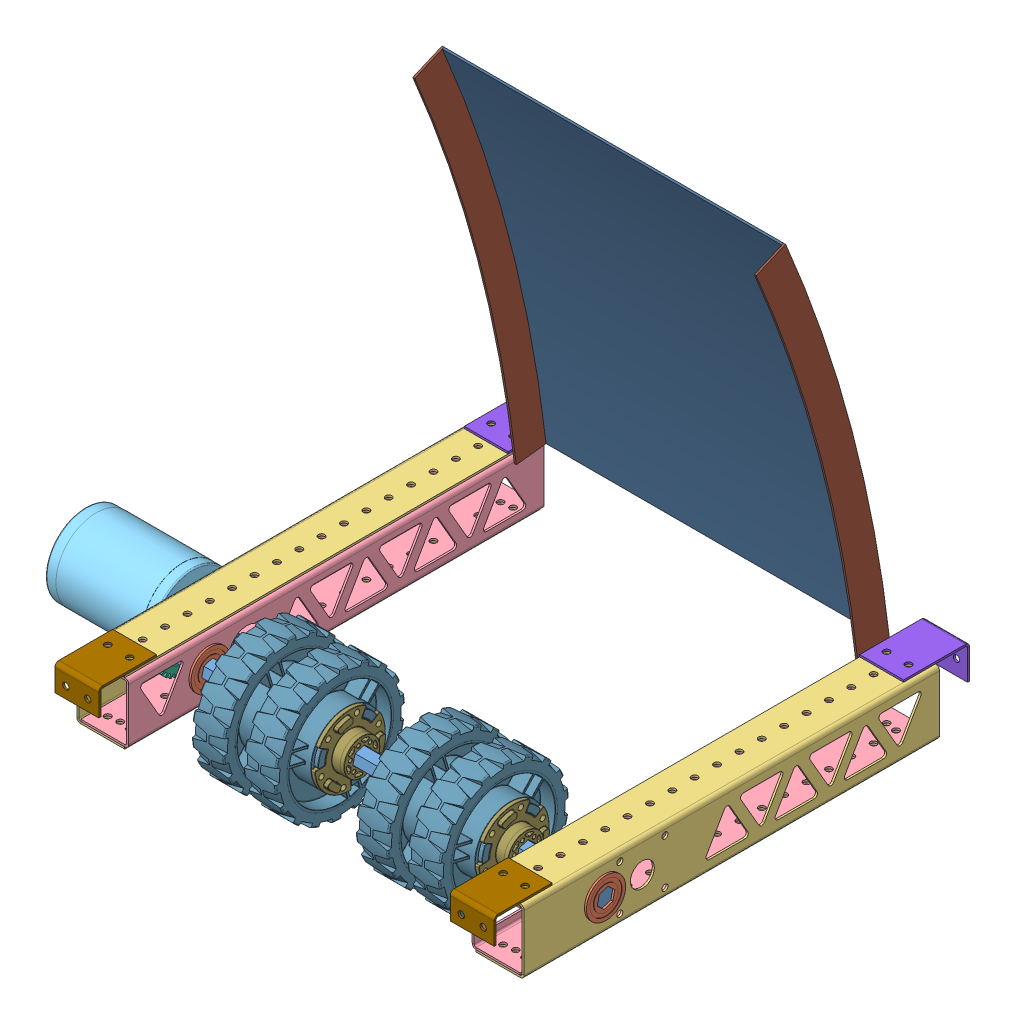
SolidWorks assembly 0001 - 03 - 1001 REVISED SHOOTER, configuration Default. Lengths in mm.
34 component instances, 15 part files, 27 mates.
Components (placement in the parent):
- 0001 - 03 - 1000 SHOOTER-1: 0001 - 03 - 1000 SHOOTER [Default] at (243.3681 260.9719 308.2005) size (448.99 90.52 330.2)
  - 0001 - 03 - 0001 Reference Geometry-1: 0001 - 03 - 0001 Reference Geometry [Default] at origin
  - 0001 - 03 - 1011 Hex Shaft-1: 0001 - 03 - 1011 Hex Shaft [Default] at (158.75 29.2246 103.7425) x (1 0 0) z (0 -0.904809 0.425818) size (355.6 13.95 14.34)
  - Hex Bearing-4: Hex Bearing [Default] at (330.2 0 101.6) x (0 -0.973926 0.226866) z (0 0.226866 0.973926) size (31.12 7.94 31.12)
  - Hex Bearing-5: Hex Bearing [Default] at (301.625 0 101.6) x (0 0.290491 -0.956878) z (0 0.956878 0.290491) size (31.12 7.94 31.12)
  - 0001 - 03 - 1023 Left Side-1: 0001 - 03 - 1023 Left Side [Default] x (0 0 1) z (-1 0 0) size (330.2 50.8 38.1)
  - 0001 - 03 - 1022 Right Side-1: 0001 - 03 - 1022 Right Side [Default] at (2.3813 0 0) x (0 0 -1) z (1 0 0) size (330.2 47.62 38.1)
  - 0001 - 03 - 1022 Right Side-2: 0001 - 03 - 1022 Right Side [Default] at (315.1187 0 0) x (0 0 -1) z (-1 0 0) size (330.2 47.62 38.1)
  - 0001 - 03 - 1023 Left Side-2: 0001 - 03 - 1023 Left Side [Default] at (317.5 0 0) x (0 0 1) z (1 0 0) size (330.2 50.8 38.1)
  - Mini-CIM-2: Mini-CIM [Default] at (-20.6375 0 71.12) x (-1 0 0) z (0 -0.707107 0.707107) size (125.82 64.01 64.01)
  - Hex Bearing-6: Hex Bearing [Default] at (-12.7 0 101.6) x (0 -0.973926 0.226866) z (0 -0.226866 -0.973926) size (31.12 7.94 31.12)
  - Hex Bearing-7: Hex Bearing [Default] at (15.875 0 101.6) x (0 0.973926 -0.226866) z (0 -0.226866 -0.973926) size (31.12 7.94 31.12)
  - 24t Vex Gear-1: 24t Vex Gear [Default] at (-6.3754 0 71.12) x (0 -0.442832 0.896605) z (-1 0 0) size (32.86 32.86 12.65)
  - 24t Vex Gear-2: 24t Vex Gear [Default] at (-6.3754 0 101.6) x (0 -0.944341 0.328968) z (-1 0 0) size (32.86 32.86 12.65)
  - CIM Shaft Adapter-1: CIM Shaft Adapter [Default] at (-16.6375 0 71.12) x (1 0 0) z (0 0.064799 0.997898) size (19.05 12.7 14.66)
- 0001 - 03 - 1024 Bracket-1: 0001 - 03 - 1024 Bracket [Default] at (244.9556 260.9719 117.7005) x (-1 0 0) z (0 0 -1) size (34.92 26.99 52.39)
- 0001 - 03 - 1024 Bracket-2: 0001 - 03 - 1024 Bracket [Default] at (559.2806 260.9719 117.7005) x (-1 0 0) z (0 0 -1) size (34.92 26.99 52.39)
- 0001 - 03 - 1025 Small Bracket-1: 0001 - 03 - 1025 Small Bracket [Default] at (244.9556 267.3219 492.3505) size (34.92 20.64 46.04)
- 0001 - 03 - 1025 Small Bracket-2: 0001 - 03 - 1025 Small Bracket [Default] at (559.2806 267.3219 492.3505) size (34.92 20.64 46.04)
- 0001 - 03 - 1026 Hood-1: 0001 - 03 - 1026 Hood [Default] at (537.0556 283.3795 141.5236) x (-1 0 0) z (0 0.115024 -0.993363) size (269.88 320.68 47.56)
- 0001 - 03 - 1027 Hood Support-1: 0001 - 03 - 1027 Hood Support [Default] at (267.1806 596.6307 224.1409) x (1 0 0) z (0 0.389841 -0.920882) size (1.59 320.68 70.41)
- 0001 - 03 - 1027 Hood Support-2: 0001 - 03 - 1027 Hood Support [Default] at (538.6431 596.6307 224.1409) x (1 0 0) z (0 0.389841 -0.920882) size (1.59 320.68 70.41)
- 0001 - 03 - 1030 WHEEL ASSEMBLY-1: 0001 - 03 - 1030 WHEEL ASSEMBLY [Default] at (328.3429 264.0107 383.1758) x (0 0.956878 0.290491) z (1 0 0) size (140.96 140.96 101.35)
  - VersaHub-1: VersaHub [Default] at (4.8265 26.3593 48.1847) size (54.75 55.87 12.7)
  - VersaThing-1: VersaThing [Default] at (4.8265 26.3593 8.6242) x (-0.5 0.866025 0) z (0.866025 0.5 0) size (55.88 12.7 55.88)
  - VEX Wheel 4in DT-1: VEX Wheel 4in DT [Default] at (4.8265 26.3593 29.1982) x (0.5 -0.866025 0) z (0 0 1) size (103.19 103.19 41.15)
  - VersaHub-2: VersaHub [Default] at (4.8265 26.3593 -30.9363) x (-0.5 -0.866025 0) z (0 0 -1) size (54.75 55.87 12.7)
  - VEX Wheel 4in DT-2: VEX Wheel 4in DT [Default] at (4.8265 26.3593 -11.9498) size (103.19 103.19 41.15)
- 0001 - 03 - 1030 WHEEL ASSEMBLY-2: 0001 - 03 - 1030 WHEEL ASSEMBLY [Default] at (475.8933 246.4805 387.2593) x (0 -0.730012 0.683435) z (-1 0 0) size (140.96 140.96 101.35)
  - VersaHub-1: VersaHub [Default] at (4.8265 26.3593 48.1847) size (54.75 55.87 12.7)
  - VersaThing-1: VersaThing [Default] at (4.8265 26.3593 8.6242) x (-0.5 0.866025 0) z (0.866025 0.5 0) size (55.88 12.7 55.88)
  - VEX Wheel 4in DT-1: VEX Wheel 4in DT [Default] at (4.8265 26.3593 29.1982) x (0.5 -0.866025 0) z (0 0 1) size (103.19 103.19 41.15)
  - VersaHub-2: VersaHub [Default] at (4.8265 26.3593 -30.9363) x (-0.5 -0.866025 0) z (0 0 -1) size (54.75 55.87 12.7)
  - VEX Wheel 4in DT-2: VEX Wheel 4in DT [Default] at (4.8265 26.3593 -11.9498) size (103.19 103.19 41.15)
Mates (geometry in assembly coordinates):
- Distance1: distance = 25.4 mm anti-aligned: plane of 0001 - 03 - 1024 Bracket-2 through (576.7431 260.9719 117.7005) normal (0 0 1); plane of 0001 - 03 - 1000 SHOOTER-1/0001 - 03 - 1022 Right Side-2 through (538.6431 281.6094 143.1005) normal (0 0 -1)
- Coincident2: coincident anti-aligned: plane of 0001 - 03 - 1000 SHOOTER-1/0001 - 03 - 1023 Left Side-2 through (579.9181 286.3719 473.3005) normal (0 1 0); plane of 0001 - 03 - 1024 Bracket-2 through (576.7431 286.3719 117.7005) normal (0 -1 0)
- Coincident3: coincident aligned: plane of 0001 - 03 - 1000 SHOOTER-1/0001 - 03 - 1022 Right Side-2 through (576.7431 283.1969 143.1005) normal (1 0 0); plane of 0001 - 03 - 1024 Bracket-2 through (576.7431 284.7844 116.113) normal (1 0 0)
- Distance2: distance = 25.4 mm anti-aligned: plane of 0001 - 03 - 1000 SHOOTER-1/0001 - 03 - 1022 Right Side-1 through (262.4181 284.7844 143.1005) normal (0 0 -1); plane of 0001 - 03 - 1024 Bracket-1 through (262.4181 260.9719 117.7005) normal (0 0 1)
- Coincident5: coincident anti-aligned: plane of 0001 - 03 - 1000 SHOOTER-1/0001 - 03 - 1023 Left Side-1 through (224.3181 286.3719 473.3005) normal (0 1 0); plane of 0001 - 03 - 1024 Bracket-1 through (262.4181 286.3719 117.7005) normal (0 -1 0)
- Coincident6: coincident aligned: plane of 0001 - 03 - 1000 SHOOTER-1/0001 - 03 - 1023 Left Side-1 through (262.4181 286.3719 473.3005) normal (1 0 0); plane of 0001 - 03 - 1024 Bracket-1 through (262.4181 284.7844 116.113) normal (1 0 0)
- Concentric1: concentric anti-aligned: cylinder of 0001 - 03 - 1000 SHOOTER-1/0001 - 03 - 1023 Left Side-2 through (568.0119 286.3719 460.6005) axis (0 -1 0) radius 2.54; cylinder of 0001 - 03 - 1025 Small Bracket-2 through (568.0119 286.3719 460.6005) axis (0 1 0) radius 2.54
- Coincident7: coincident anti-aligned: plane of 0001 - 03 - 1000 SHOOTER-1/0001 - 03 - 1023 Left Side-2 through (579.9181 286.3719 473.3005) normal (0 1 0); plane of 0001 - 03 - 1025 Small Bracket-2 through (541.8181 286.3719 492.3505) normal (0 -1 0)
- Concentric2: concentric anti-aligned: cylinder of 0001 - 03 - 1000 SHOOTER-1/0001 - 03 - 1023 Left Side-2 through (550.5494 286.3719 460.6005) axis (0 -1 0) radius 2.54; cylinder of 0001 - 03 - 1025 Small Bracket-2 through (550.5494 286.3719 460.6005) axis (0 1 0) radius 2.54
- Concentric3: concentric aligned: cylinder of 0001 - 03 - 1000 SHOOTER-1/0001 - 03 - 1023 Left Side-1 through (253.6869 235.5719 460.6005) axis (0 1 0) radius 2.54; cylinder of 0001 - 03 - 1025 Small Bracket-1 through (253.6869 286.3719 460.6005) axis (0 1 0) radius 2.54
- Concentric4: concentric aligned: cylinder of 0001 - 03 - 1000 SHOOTER-1/0001 - 03 - 1023 Left Side-1 through (236.2244 235.5719 460.6005) axis (0 1 0) radius 2.54; cylinder of 0001 - 03 - 1025 Small Bracket-1 through (236.2244 286.3719 460.6005) axis (0 1 0) radius 2.54
- Coincident8: coincident anti-aligned: plane of 0001 - 03 - 1000 SHOOTER-1/0001 - 03 - 1023 Left Side-1 through (224.3181 286.3719 473.3005) normal (0 1 0); plane of 0001 - 03 - 1025 Small Bracket-1 through (227.4931 286.3719 492.3505) normal (0 -1 0)
- Coincident10: coincident: plane of 0001 - 03 - 1000 SHOOTER-1/0001 - 03 - 1022 Right Side-1 through (262.4181 240.3344 143.1005) normal (0 0 -1); line of 0001 - 03 - 1026 Hood-1 through (267.1806 283.1969 143.1005) axis (1 0 0)
- Coincident12: coincident: line of 0001 - 03 - 1000 SHOOTER-1/0001 - 03 - 1022 Right Side-2 through (541.8181 283.1969 143.1005) axis (1 0 0); plane of 0001 - 03 - 1026 Hood-1 through (267.1806 283.1969 143.1005) normal (0 -0.972217 -0.234083)
- Concentric8: concentric aligned: cylinder of 0001 - 03 - 1026 Hood-1 through (267.1806 16.7487 1249.7406) axis (1 0 0) radius 1139.8524; cylinder of 0001 - 03 - 1027 Hood Support-1 through (265.5931 16.7487 1249.7406) axis (1 0 0) radius 1139.8524
- Coincident13: coincident anti-aligned: plane of 0001 - 03 - 1026 Hood-1 through (267.1806 16.7487 1249.7406) normal (-1 0 0); plane of 0001 - 03 - 1027 Hood Support-1 through (267.1806 16.7487 1249.7406) normal (1 0 0)
- Coincident14: coincident anti-aligned: circle of 0001 - 03 - 1000 SHOOTER-1/0001 - 03 - 1022 Right Side-1; plane of 0001 - 03 - 1027 Hood Support-1 through (265.5931 16.7487 1249.7406) normal (-1 0 0)
- Coincident15: coincident aligned: plane of 0001 - 03 - 1026 Hood-1 through (267.1806 283.1969 143.1005) normal (0 -0.972217 -0.234083); plane of 0001 - 03 - 1027 Hood Support-1 through (265.5931 277.6228 166.2514) normal (0 -0.972217 -0.234083)
- Concentric9: concentric aligned: cylinder of 0001 - 03 - 1026 Hood-1 through (267.1806 16.7487 1249.7406) axis (1 0 0) radius 1139.8524; cylinder of 0001 - 03 - 1027 Hood Support-2 through (537.0556 16.7487 1249.7406) axis (1 0 0) radius 1139.8524
- Coincident17: coincident aligned: plane of 0001 - 03 - 1026 Hood-1 through (267.1806 283.1969 143.1005) normal (0 -0.972217 -0.234083); plane of 0001 - 03 - 1027 Hood Support-2 through (537.0556 277.6228 166.2514) normal (0 -0.972217 -0.234083)
- Coincident18: coincident anti-aligned: plane of 0001 - 03 - 1026 Hood-1 through (537.0556 16.7487 1249.7406) normal (1 0 0); plane of 0001 - 03 - 1027 Hood Support-2 through (537.0556 16.7487 1249.7406) normal (-1 0 0)
- Concentric10: concentric anti-aligned: cylinder of 0001 - 03 - 1000 SHOOTER-1/Hex Bearing-7 through (259.2431 260.9719 409.8005) axis (1 0 0) radius 15.5575; cylinder of 0001 - 03 - 1030 WHEEL ASSEMBLY-1/VersaHub-1 through (387.6401 260.9719 409.8005) axis (-1 0 0) radius 14.3002
- Concentric11: concentric anti-aligned: cone of 0001 - 03 - 1030 WHEEL ASSEMBLY-1/VEX Wheel 4in DT-1 through (358.8385 260.9719 409.8005) axis (1 0 0); cone of 0001 - 03 - 1030 WHEEL ASSEMBLY-2/VEX Wheel 4in DT-1 through (445.3977 260.9719 409.8005) axis (-1 0 0)
- Distance3: distance = 38.1 mm anti-aligned: plane of 0001 - 03 - 1030 WHEEL ASSEMBLY-1/VEX Wheel 4in DT-2 through (303.6931 220.4107 397.4868) normal (-1 0 0); plane of 0001 - 03 - 1000 SHOOTER-1/0001 - 03 - 1022 Right Side-1 through (265.5931 283.1969 143.1005) normal (1 0 0)
- Distance4: distance = 38.1 mm anti-aligned: plane of 0001 - 03 - 1030 WHEEL ASSEMBLY-2/VEX Wheel 4in DT-2 through (500.5431 291.9165 380.8303) normal (1 0 0); plane of 0001 - 03 - 1000 SHOOTER-1/0001 - 03 - 1022 Right Side-2 through (538.6431 238.7469 143.1005) normal (-1 0 0)
- Concentric12: concentric anti-aligned: cylinder of 0001 - 03 - 1030 WHEEL ASSEMBLY-1/VersaHub-1 through (374.9401 284.1635 404.3983) axis (1 0 0) radius 2.1526; cylinder of 0001 - 03 - 1030 WHEEL ASSEMBLY-2/VersaHub-1 through (429.2961 284.1635 404.3983) axis (-1 0 0) radius 2.1526
- Coincident24: coincident anti-aligned: plane of 0001 - 03 - 1000 SHOOTER-1/0001 - 03 - 1011 Hex Shaft-1 through (224.3181 268.1131 408.1371) normal (0 0.956878 0.290491); plane of 0001 - 03 - 1030 WHEEL ASSEMBLY-2/VersaHub-1 through (416.5961 268.1131 408.1371) normal (0 -0.956878 -0.290491)
